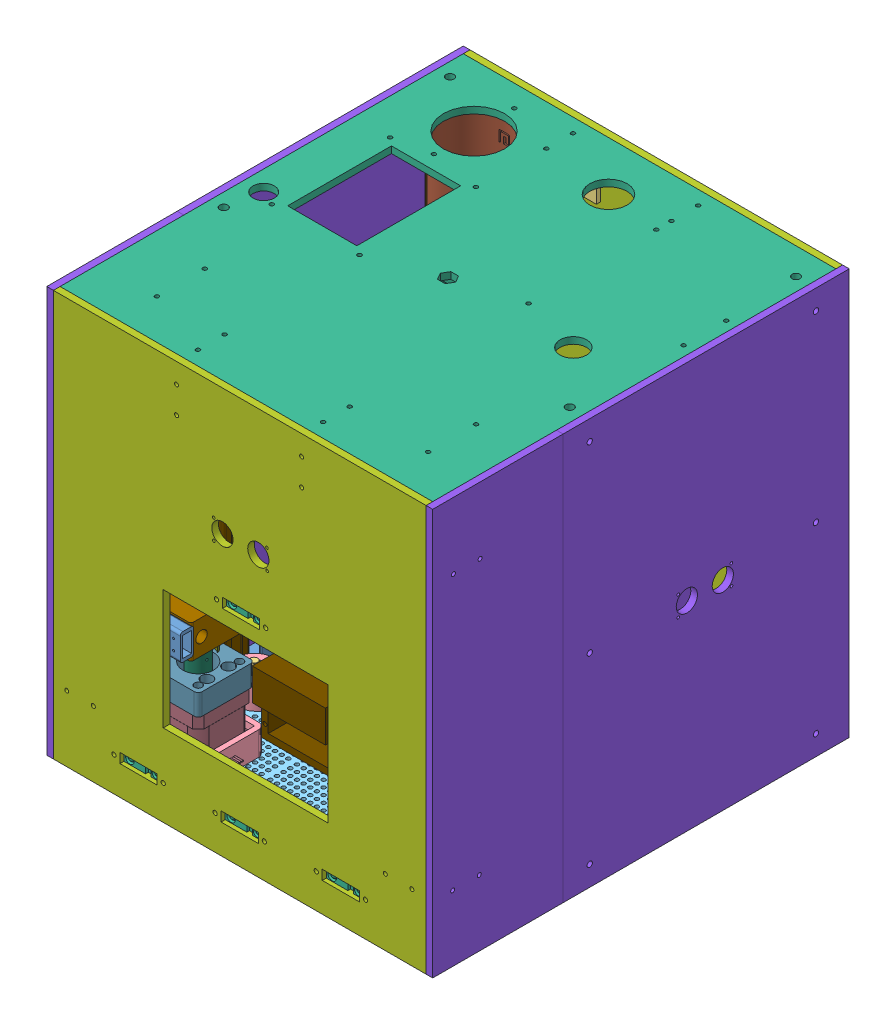
SolidWorks assembly Base_grand_robot_V3, configuration Défaut. Lengths in mm.
Overall size (315.25 345.84 313).
174 component instances, 54 part files, 167 mates.
Components (placement in the parent):
- base_v3-1: base_v3 [Défaut] at (-13.7179 5.8501 0) size (280 5 210)
- bille_porteuse-1: bille_porteuse [Défaut] at (91.4296 18.7222 119.3)
- bille_porteuse-3: bille_porteuse [Défaut] at (-113.9704 18.7222 119.3)
- bille_porteuse-4: bille_porteuse [Défaut] at (91.4296 18.7222 89.3)
- bloc moteur-1: bloc moteur [Défaut] at (-93.812 100.3945 0) size (96.7 249.86 114.05)
  - support moteur-1: support moteur [Défaut] at (-52.9059 10.4555 40) size (89 2 80)
  - support central-1: support central [Défaut] at (30.0941 -89.5445 40) size (6 100 80)
  - support inter-1: support inter [Défaut] at (-10.9059 -89.5445 40) size (6 100 80)
  - support exter-1: support exter [Défaut] at (-52.9059 -27.5445 40) x (-1 0 0) z (0 -1 0) size (6 80 25)
  - RENFORT-1: RENFORT [Défaut] at (-10.9059 -27.5445 -30) x (0 0 -1) z (1 0 0) size (10 38 42)
  - RENFORT-2: RENFORT [Défaut] at (-10.9059 -27.5445 40) x (0 0 -1) z (1 0 0) size (10 38 42)
  - fix carre-1: fix carre [Défaut] at (30.0941 -89.5445 0) x (0 0 -1) z (1 0 0) size (80 10 10)
  - fix carre-2: fix carre [Défaut] at (30.0941 0.4555 0) x (0 0 1) z (0 -1 0) size (80 10 10)
  - fix carre-3: fix carre [Défaut] at (-10.9059 -89.5445 0) x (0 0 -1) z (1 0 0) size (80 10 10)
  - moteur-1: moteur [Défaut] at (-31.9059 133.2945 0.001) x (-0.000071 0 -1) z (-1 0 0.000071) size (36.98 140.84 36.98)
  - support coulisse-1: support coulisse [Défaut] at (-48.9059 -11.0445 -20) x (1 0 0) z (0 1 0) size (28 10 10)
  - support coulisse-2: support coulisse [Défaut] at (-48.9059 -11.0445 30) x (1 0 0) z (0 1 0) size (28 10 10)
  - axe inter-1: axe inter [Défaut] at (36.0941 -12.5445 0) x (0 0.999221 -0.039455) z (-1 0 0) size (8 8 60)
  - axe roue-1: axe roue [Défaut] at (36.0941 -59.5445 0) x (0 0.572266 -0.820068) z (-1 0 0) size (8 8 50)
  - roue-1: roue [Défaut] at (5.7816 -59.5445 0) x (0 -0.770299 0.637683) z (0 -0.637683 -0.770299) size (81 21.5 81)
  - angular contact ball bearing_68_iso-6: angular contact ball bearing_68_iso [ISO 15 ABB - 288 - 12,SI,NC,12_68] at (-7.4059 -12.5445 0) size (5 16 16)
  - angular contact ball bearing_68_iso-7: angular contact ball bearing_68_iso [ISO 15 ABB - 288 - 12,SI,NC,12_68] at (33.5941 -59.5445 0) size (5 16 16)
  - angular contact ball bearing_68_iso-8: angular contact ball bearing_68_iso [ISO 15 ABB - 288 - 12,SI,NC,12_68] at (-55.4059 -12.5445 0) x (-1 0 0) z (0 0.924225 0.381849) size (5 16 16)
  - angular contact ball bearing_68_iso-9: angular contact ball bearing_68_iso [ISO 15 ABB - 288 - 12,SI,NC,12_68] at (-8.4059 -59.5445 0) size (5 16 16)
  - angular contact ball bearing_68_iso-10: angular contact ball bearing_68_iso [ISO 15 ABB - 288 - 12,SI,NC,12_68] at (33.5941 -12.5445 0) x (1 0 0) z (0 0.752289 -0.658833) size (5 16 16)
  - poulie 20 dents-1: poulie 20 dents [Défaut] at (19.2816 -12.5445 0) x (0 -0.673947 -0.73878) z (1 0 0) size (24 24 16.81)
  - poulie 30 dents-1: poulie 30 dents [Défaut] at (28.2816 -59.5445 0) x (0 -0.380704 -0.924697) z (-1 0 0) size (28.16 28.16 8)
  - Courroie2^bloc moteur-1: Courroie2^bloc moteur [Défaut] at (28.2816 -59.5445 0) x (0 0 -1) z (1 0 0) size (30.24 72.47 0) (virtual)
  - socket head cap screw_iso-1: socket head cap screw_iso [ISO 4762 M5 x 16 --- 16C] at (-47.9059 15.6555 35) x (0 -1 0) z (0.408943 0 0.91256) size (21 8.5 8.5)
  - socket head cap screw_iso-2: socket head cap screw_iso [ISO 4762 M5 x 16 --- 16C] at (-47.9059 15.6555 -35) x (0 -1 0) z (1 0 0) size (21 8.5 8.5)
  - socket head cap screw_iso-3: socket head cap screw_iso [ISO 4762 M5 x 16 --- 16C] at (-15.9059 15.6555 -35) x (0 -1 0) z (-0.986774 0 0.1621) size (21 8.5 8.5)
  - socket head cap screw_iso-4: socket head cap screw_iso [ISO 4762 M5 x 16 --- 16C] at (-15.9059 15.6555 35) x (0 -1 0) z (0 0 1) size (21 8.5 8.5)
  - socket head cap screw_iso-5: socket head cap screw_iso [ISO 4762 M6 x 10 --- 10C] at (25.0941 16.7055 -20) x (0 -1 0) z (0.924225 0 -0.381849) size (16 10 10)
  - socket head cap screw_iso-6: socket head cap screw_iso [ISO 4762 M6 x 10 --- 10C] at (25.0941 16.7055 20) x (0 -1 0) z (0 0 1) size (16 10 10)
  - socket head cap screw_iso-7: socket head cap screw_iso [ISO 4762 M6 x 16 --- 16C] at (-43.9059 -16.0445 -46.25) x (0 0 1) z (-1 0 0) size (22 10 10)
  - socket head cap screw_iso-8: socket head cap screw_iso [ISO 4762 M6 x 16 --- 16C] at (-25.9059 -16.0445 -46.25) x (0 0 1) z (-1 0 0) size (22 10 10)
  - socket head cap screw_iso-9: socket head cap screw_iso [ISO 4762 M6 x 16 --- 16C] at (-43.9059 -16.0445 46.25) x (0 0 -1) z (-0.381849 0.924225 0) size (22 10 10)
  - socket head cap screw_iso-10: socket head cap screw_iso [ISO 4762 M6 x 16 --- 16C] at (-25.9059 -16.0445 46.25) x (0 0 -1) z (0.987997 0.154474 0) size (22 10 10)
  - socket countersunk head screw_iso-1: socket countersunk head screw_iso [ISO 10642 - M5 x 16 --- 16N] at (-60.0059 -9.5445 35) x (1 0 0) z (0 -0.519107 0.854709) size (16 9.43 9.43)
  - socket countersunk head screw_iso-2: socket countersunk head screw_iso [ISO 10642 - M5 x 16 --- 16N] at (-60.0059 -22.5445 35) size (16 9.43 9.43)
  - socket countersunk head screw_iso-3: socket countersunk head screw_iso [ISO 10642 - M5 x 16 --- 16N] at (-60.0059 -22.5445 -35) size (16 9.43 9.43)
  - socket countersunk head screw_iso-4: socket countersunk head screw_iso [ISO 10642 - M5 x 16 --- 16N] at (-60.0059 -9.5445 -35) x (1 0 0) z (0 0.039879 0.999205) size (16 9.43 9.43)
  - socket countersunk head screw_iso-5: socket countersunk head screw_iso [ISO 10642 - M5 x 16 --- 16N] at (36.6941 5.4555 30) x (-1 0 0) z (0 0.924225 0.381849) size (16 9.43 9.43)
  - socket countersunk head screw_iso-6: socket countersunk head screw_iso [ISO 10642 - M5 x 16 --- 16N] at (36.6941 5.4555 -30) x (-1 0 0) z (0 0.924225 0.381849) size (16 9.43 9.43)
  - socket countersunk head screw_iso-7: socket countersunk head screw_iso [ISO 10642 - M5 x 16 --- 16N] at (36.6941 -84.5445 20) x (-1 0 0) z (0 0.924225 0.381849) size (16 9.43 9.43)
  - socket countersunk head screw_iso-8: socket countersunk head screw_iso [ISO 10642 - M5 x 16 --- 16N] at (36.6941 -84.5445 -20) x (-1 0 0) z (0 0.924225 0.381849) size (16 9.43 9.43)
  - socket countersunk head screw_iso-10: socket countersunk head screw_iso [ISO 10642 - M5 x 16 --- 16N] at (-4.3059 -84.5445 20) x (-1 0 0) z (0 0.924225 0.381849) size (16 9.43 9.43)
- bloc moteur-2: bloc moteur [Défaut] at (66.3761 100.3945 0) x (-1 0 0) z (0 0 -1) size (96.7 249.86 114.05)
  - support moteur-1: support moteur [Défaut] at (-52.9059 10.4555 40) size (89 2 80)
  - support central-1: support central [Défaut] at (30.0941 -89.5445 40) size (6 100 80)
  - support inter-1: support inter [Défaut] at (-10.9059 -89.5445 40) size (6 100 80)
  - support exter-1: support exter [Défaut] at (-52.9059 -27.5445 40) x (-1 0 0) z (0 -1 0) size (6 80 25)
  - RENFORT-1: RENFORT [Défaut] at (-10.9059 -27.5445 -30) x (0 0 -1) z (1 0 0) size (10 38 42)
  - RENFORT-2: RENFORT [Défaut] at (-10.9059 -27.5445 40) x (0 0 -1) z (1 0 0) size (10 38 42)
  - fix carre-1: fix carre [Défaut] at (30.0941 -89.5445 0) x (0 0 -1) z (1 0 0) size (80 10 10)
  - fix carre-2: fix carre [Défaut] at (30.0941 0.4555 0) x (0 0 1) z (0 -1 0) size (80 10 10)
  - fix carre-3: fix carre [Défaut] at (-10.9059 -89.5445 0) x (0 0 -1) z (1 0 0) size (80 10 10)
  - moteur-1: moteur [Défaut] at (-31.9059 133.2945 0.001) x (-0.000071 0 -1) z (-1 0 0.000071) size (36.98 140.84 36.98)
  - support coulisse-1: support coulisse [Défaut] at (-48.9059 -11.0445 -20) x (1 0 0) z (0 1 0) size (28 10 10)
  - support coulisse-2: support coulisse [Défaut] at (-48.9059 -11.0445 30) x (1 0 0) z (0 1 0) size (28 10 10)
  - axe inter-1: axe inter [Défaut] at (36.0941 -12.5445 0) x (0 0.999221 -0.039455) z (-1 0 0) size (8 8 60)
  - axe roue-1: axe roue [Défaut] at (36.0941 -59.5445 0) x (0 0.572266 -0.820068) z (-1 0 0) size (8 8 50)
  - roue-1: roue [Défaut] at (5.7816 -59.5445 0) x (0 -0.770299 0.637683) z (0 -0.637683 -0.770299) size (81 21.5 81)
  - angular contact ball bearing_68_iso-6: angular contact ball bearing_68_iso [ISO 15 ABB - 288 - 12,SI,NC,12_68] at (-7.4059 -12.5445 0) size (5 16 16)
  - angular contact ball bearing_68_iso-7: angular contact ball bearing_68_iso [ISO 15 ABB - 288 - 12,SI,NC,12_68] at (33.5941 -59.5445 0) size (5 16 16)
  - angular contact ball bearing_68_iso-8: angular contact ball bearing_68_iso [ISO 15 ABB - 288 - 12,SI,NC,12_68] at (-55.4059 -12.5445 0) x (-1 0 0) z (0 0.924225 0.381849) size (5 16 16)
  - angular contact ball bearing_68_iso-9: angular contact ball bearing_68_iso [ISO 15 ABB - 288 - 12,SI,NC,12_68] at (-8.4059 -59.5445 0) size (5 16 16)
  - angular contact ball bearing_68_iso-10: angular contact ball bearing_68_iso [ISO 15 ABB - 288 - 12,SI,NC,12_68] at (33.5941 -12.5445 0) x (1 0 0) z (0 0.752289 -0.658833) size (5 16 16)
  - poulie 20 dents-1: poulie 20 dents [Défaut] at (19.2816 -12.5445 0) x (0 -0.673947 -0.73878) z (1 0 0) size (24 24 16.81)
  - poulie 30 dents-1: poulie 30 dents [Défaut] at (28.2816 -59.5445 0) x (0 -0.380704 -0.924697) z (-1 0 0) size (28.16 28.16 8)
  - Courroie2^bloc moteur-1: Courroie2^bloc moteur [Défaut] at (28.2816 -59.5445 0) x (0 0 -1) z (1 0 0) size (30.24 72.47 0) (virtual)
  - socket head cap screw_iso-1: socket head cap screw_iso [ISO 4762 M5 x 16 --- 16C] at (-47.9059 15.6555 35) x (0 -1 0) z (0.408943 0 0.91256) size (21 8.5 8.5)
  - socket head cap screw_iso-2: socket head cap screw_iso [ISO 4762 M5 x 16 --- 16C] at (-47.9059 15.6555 -35) x (0 -1 0) z (1 0 0) size (21 8.5 8.5)
  - socket head cap screw_iso-3: socket head cap screw_iso [ISO 4762 M5 x 16 --- 16C] at (-15.9059 15.6555 -35) x (0 -1 0) z (-0.986774 0 0.1621) size (21 8.5 8.5)
  - socket head cap screw_iso-4: socket head cap screw_iso [ISO 4762 M5 x 16 --- 16C] at (-15.9059 15.6555 35) x (0 -1 0) z (0 0 1) size (21 8.5 8.5)
  - socket head cap screw_iso-5: socket head cap screw_iso [ISO 4762 M6 x 10 --- 10C] at (25.0941 16.7055 -20) x (0 -1 0) z (0.924225 0 -0.381849) size (16 10 10)
  - socket head cap screw_iso-6: socket head cap screw_iso [ISO 4762 M6 x 10 --- 10C] at (25.0941 16.7055 20) x (0 -1 0) z (0 0 1) size (16 10 10)
  - socket head cap screw_iso-7: socket head cap screw_iso [ISO 4762 M6 x 16 --- 16C] at (-43.9059 -16.0445 -46.25) x (0 0 1) z (-1 0 0) size (22 10 10)
  - socket head cap screw_iso-8: socket head cap screw_iso [ISO 4762 M6 x 16 --- 16C] at (-25.9059 -16.0445 -46.25) x (0 0 1) z (-1 0 0) size (22 10 10)
  - socket head cap screw_iso-9: socket head cap screw_iso [ISO 4762 M6 x 16 --- 16C] at (-43.9059 -16.0445 46.25) x (0 0 -1) z (-0.381849 0.924225 0) size (22 10 10)
  - socket head cap screw_iso-10: socket head cap screw_iso [ISO 4762 M6 x 16 --- 16C] at (-25.9059 -16.0445 46.25) x (0 0 -1) z (0.987997 0.154474 0) size (22 10 10)
  - socket countersunk head screw_iso-1: socket countersunk head screw_iso [ISO 10642 - M5 x 16 --- 16N] at (-60.0059 -9.5445 35) x (1 0 0) z (0 -0.519107 0.854709) size (16 9.43 9.43)
  - socket countersunk head screw_iso-2: socket countersunk head screw_iso [ISO 10642 - M5 x 16 --- 16N] at (-60.0059 -22.5445 35) size (16 9.43 9.43)
  - socket countersunk head screw_iso-3: socket countersunk head screw_iso [ISO 10642 - M5 x 16 --- 16N] at (-60.0059 -22.5445 -35) size (16 9.43 9.43)
  - socket countersunk head screw_iso-4: socket countersunk head screw_iso [ISO 10642 - M5 x 16 --- 16N] at (-60.0059 -9.5445 -35) x (1 0 0) z (0 0.039879 0.999205) size (16 9.43 9.43)
  - socket countersunk head screw_iso-5: socket countersunk head screw_iso [ISO 10642 - M5 x 16 --- 16N] at (36.6941 5.4555 30) x (-1 0 0) z (0 0.924225 0.381849) size (16 9.43 9.43)
  - socket countersunk head screw_iso-6: socket countersunk head screw_iso [ISO 10642 - M5 x 16 --- 16N] at (36.6941 5.4555 -30) x (-1 0 0) z (0 0.924225 0.381849) size (16 9.43 9.43)
  - socket countersunk head screw_iso-7: socket countersunk head screw_iso [ISO 10642 - M5 x 16 --- 16N] at (36.6941 -84.5445 20) x (-1 0 0) z (0 0.924225 0.381849) size (16 9.43 9.43)
  - socket countersunk head screw_iso-8: socket countersunk head screw_iso [ISO 10642 - M5 x 16 --- 16N] at (36.6941 -84.5445 -20) x (-1 0 0) z (0 0.924225 0.381849) size (16 9.43 9.43)
  - socket countersunk head screw_iso-10: socket countersunk head screw_iso [ISO 10642 - M5 x 16 --- 16N] at (-4.3059 -84.5445 20) x (-1 0 0) z (0 0.924225 0.381849) size (16 9.43 9.43)
- socket countersunk head screw_iso-10: socket countersunk head screw_iso [ISO 10642 - M5 x 16 --- 16N] at (82.2821 24.0329 -30) x (0 -1 0) z (-0.068023 0 0.997684) size (16 9.43 9.43)
- Profile-1: Profile [Défaut] at (-133.7179 310.8501 75) x (1 0 0) z (0 -1 0) size (20 20 300)
- Profile-2: Profile [Défaut] at (126.2821 310.8501 75) x (1 0 0) z (0 -1 0) size (20 20 300)
- bille-1: bille [Défaut] at (88.9821 9.4556 -89.3) size (14 14 14)
- porte_bille-1: porte_bille [Défaut] at (88.9821 9.4556 -89.3) size (16 1.79 16)
- contour_roulement-1: contour_roulement [Défaut] at (88.9821 22.8501 -89.3) x (0.737581 0 0.675259) z (-0.675259 0 0.737581) size (20 32.58 20)
- bille_porteuse-5: bille_porteuse [Défaut] at (-113.9704 18.7222 -119.3)
- Support_bille_appui-1: Support_bille_appui [Défaut] at (88.9821 10.8501 -89.3) x (0 0 1) z (-1 0 0) size (30 20 30)
- ecrou socket-1: ecrou socket [Défaut] at (88.9821 33.8501 -89.3) x (1 0 0) z (0 -1 0) size (12.41 10.75 3)
- ecrou socket-2: ecrou socket [Défaut] at (-116.4179 33.8501 89.3) x (1 0 0) z (0 -1 0) size (12.41 10.75 3)
- ecrou socket-3: ecrou socket [Défaut] at (-116.4179 33.8501 -89.3) x (1 0 0) z (0 -1 0) size (12.41 10.75 3)
- ecrou socket-4: ecrou socket [Défaut] at (88.9821 33.8501 89.3) x (1 0 0) z (0 -1 0) size (12.41 10.75 3)
- bille-2: bille [Défaut] at (-116.4179 9.4556 -89.3) size (14 14 14)
- bille-3: bille [Défaut] at (88.9821 9.4556 89.3) size (14 14 14)
- bille-4: bille [Défaut] at (-116.4179 9.4556 89.3) size (14 14 14)
- contour_roulement-2: contour_roulement [Défaut] at (-116.4179 21.8501 89.3) size (20 32.58 20)
- contour_roulement-3: contour_roulement [Défaut] at (-116.4179 21.8501 -89.3) size (20 32.58 20)
- contour_roulement-4: contour_roulement [Défaut] at (88.9821 21.8501 89.3) size (20 32.58 20)
- Support_bille_appui-2: Support_bille_appui [Défaut] at (-116.4179 10.8501 -89.3) size (30 20 30)
- Support_bille_appui-3: Support_bille_appui [Défaut] at (88.9821 10.8501 89.3) size (30 20 30)
- Support_bille_appui-4: Support_bille_appui [Défaut] at (-116.4179 10.8501 89.3) size (30 20 30)
- Profile-3: Profile [Défaut] at (-133.7179 310.8501 -95) x (1 0 0) z (0 -1 0) size (20 20 300)
- Profile-4: Profile [Défaut] at (126.2821 310.8501 -95) x (1 0 0) z (0 -1 0) size (20 20 300)
- porte_bille-2: porte_bille [Défaut] at (-116.4179 9.4556 -89.3) size (16 1.79 16)
- porte_bille-3: porte_bille [Défaut] at (-116.4179 9.4556 89.3) size (16 1.79 16)
- porte_bille-4: porte_bille [Défaut] at (88.9821 9.4556 89.3) size (16 1.79 16)
- support_haut_moteur-2: support_haut_moteur [Défaut] at (-153.7179 310.8501 105) x (1 0 0) z (0 1 0) size (280 303 5)
- Protege_arriere-1: Protege_arriere [Défaut] at (-153.7179 10.8501 -110) size (280 305 5)
- Protege_laterale_gauche-1: Protege_laterale_gauche [Défaut] at (131.2821 10.8501 -110) x (0 0 1) z (-1 0 0) size (313 305 5)
- Protege_laterale_gauche-2: Protege_laterale_gauche [Défaut] at (-158.7179 315.8501 -110) x (0 0 1) z (1 0 0) size (313 305 5)
- SUPPORT DU MILIEU-1: SUPPORT DU MILIEU [Défaut] at (-112.6768 236.5001 168.8547) x (0 0 1) z (0 -1 0) size (77 260.78 291)
  - support-milieu_droite-1: support-milieu_droite [Défaut] at (-88.6499 -39.4754 108.65) size (60 77 67.3)
  - support-milieu_gauche-1: support-milieu_gauche [Défaut] at (52.3501 -167.1754 108.65) x (-1 0 0) z (0 0 1) size (65 52.31 50)
  - poulie pour courroie-2: poulie pour courroie [Défaut] at (-30.6416 -209.3078 87.41) x (0 0.720856 -0.693085) z (-1 0 0) size (14 14 16)
  - roulement lineaire M8-24-1: roulement lineaire M8-24 [Défaut] at (-27.6499 -177.1754 109.65) size (15 15 24)
  - roulement lineaire M8-24-2: roulement lineaire M8-24 [Défaut] at (-11.3499 -177.1754 109.65) size (15 15 24)
  - roulement lineaire M8-24-3: roulement lineaire M8-24 [Défaut] at (3.3501 -113.5864 121.15) x (0.720875 0 -0.693065) z (0 1 0) size (15 15 24)
  - roulement lineaire M8-24-4: roulement lineaire M8-24 [Défaut] at (-40.6499 -113.5864 121.15) x (1 0 0) z (0 1 0) size (15 15 24)
  - roulement lineaire M8-24-5: roulement lineaire M8-24 [Défaut] at (-10.6499 -29.4754 109.65) size (15 15 24)
  - roulement lineaire M8-24-6: roulement lineaire M8-24 [Défaut] at (-26.9499 -29.4808 109.65) size (15 15 24)
  - moteur NEMA 17-40mm-2: moteur NEMA 17-40mm [Défaut] at (-18.8047 -14.8331 176.65) size (42.3 52.3 64)
  - moteur NEMA 17-40mm-3: moteur NEMA 17-40mm [Défaut] at (-19.4999 -191.8089 176.65) size (42.3 52.3 64)
  - support8moteur-1: support8moteur [Défaut] at (-39.9547 -35.9831 160.65) size (42.3 42.3 16)
  - support8moteur-2: support8moteur [Défaut] at (1.6501 -170.6589 160.65) x (-1 0 0) z (0 0 1) size (42.3 42.3 16)
  - Adaptateur-1: Adaptateur [Défaut] at (-18.1766 -22.3068 142.65) x (0 0 1) z (-0.996487 -0.083748 0) size (32 15 15)
  - Adaptateur-2: Adaptateur [Défaut] at (-21.6474 -198.9949 142.65) x (0 0 1) z (-0.95813 0.286335 0) size (32 15 15)
  - PINCE_ANTI_WOOBLE-1: PINCE_ANTI_WOOBLE [Défaut] at (-19.915 -24.8562 132.474) x (0.497684 -0.867358 0) z (0 0 1) size (29.81 20 10)
  - PINCE_ANTI_WOOBLE-2: PINCE_ANTI_WOOBLE [Défaut] at (-26.86 -198.7027 133.65) x (-0.185768 -0.982594 0) z (0 0 1) size (29.81 20 10)
  - support_haut-1: support_haut [Défaut] at (8.4901 -167.1639 -59.35) x (0 -1 0) z (0 0 -1) size (47.74 55.98 15)
  - support_haut-2: support_haut [Défaut] at (-46.7865 -39.4874 -59.35) x (-0.000332 1 0) z (0 0 -1) size (47.74 55.98 15)
  - moteur NEMA 17-40mm-4: moteur NEMA 17-40mm [Défaut] at (-28.6499 16.6746 87.5) x (0 1 0) z (1 0 0) size (42.3 52.3 64)
  - poulie pour courroie-3: poulie pour courroie [Défaut] at (-30.6499 16.6746 87.5) x (0 -0.523843 -0.851815) z (-1 0 0) size (14 14 16)
  - ENSEMBLE CHARIOT DEPLACEMENT_1-1: ENSEMBLE CHARIOT DEPLACEMENT_1 [Défaut] at (-40.172 -62.0864 90.8609) x (0 0 1) z (0 -1 0) size (95 70 55)
  - support_fin_de_coursz-1: support_fin_de_coursz [Défaut] at (21.3501 -6.4754 128.814) x (-1 0 0) z (0 -1 0) size (10 20 35)
  - support_fin_de_coursz-2: support_fin_de_coursz [Défaut] at (12.3501 -200.1754 128.65) x (1 0 0) z (0 1 0) size (10 20 35)
- socle00-1: socle00 [Défaut] at (-131.7179 15.8501 -105.2) x (1 0 0) z (0 -1 0) size (236 105.2 5)
- EQUERRE-1: EQUERRE [Défaut] at (43.2821 15.8501 -105.1) x (0 1 0) z (0 0 1) size (40 20 40)
- EQUERRE-2: EQUERRE [Défaut] at (-50.7179 15.8501 -105.1) x (0 1 0) z (0 0 1) size (40 20 40)
- EQUERRE-3: EQUERRE [Défaut] at (-70.7179 310.8501 -105) x (0 -1 0) z (0 0 1) size (40 20 40)
- EQUERRE-4: EQUERRE [Défaut] at (23.2821 310.8501 -105) x (0 -1 0) z (0 0 1) size (40 20 40)
- support moteur pas a pas-1: support moteur pas a pas [Default] at (104.2821 15.8501 124.9) x (-1 0 0) z (0 1 0) size (50.3 50.3 18)
- support moteur pas a pas-2: support moteur pas a pas [Default] at (-72.6937 15.8501 124.9) x (-1 0 0) z (0 1 0) size (50.3 50.3 18)
- socleV2-1: socleV2 [Default] at (-131.7179 10.8501 105.2) x (1 0 0) z (0 1 0) size (280 175.2 5)
- Ram Electronics Shop_IR Sensor_SHARP-10: Ram Electronics Shop_IR Sensor_SHARP [Default] at (-89.7679 36.4501 186.5) x (-1 0 0) z (0 1 0) size (44.5 13.5 17.1)
- Ram Electronics Shop_IR Sensor_SHARP-11: Ram Electronics Shop_IR Sensor_SHARP [Default] at (-13.7179 36.5501 186.5) x (-1 0 0) z (0 1 0) size (44.5 13.5 17.1)
- Ram Electronics Shop_IR Sensor_SHARP-12: Ram Electronics Shop_IR Sensor_SHARP [Default] at (-12.7679 176.0501 186.5) x (-1 0 0) z (0 1 0) size (44.5 13.5 17.1)
- Ram Electronics Shop_IR Sensor_SHARP-13: Ram Electronics Shop_IR Sensor_SHARP [Default] at (62.2821 36.4501 186.5) x (-1 0 0) z (0 1 0) size (44.5 13.5 17.1)
- Ram Electronics Shop_IR Sensor_SHARP-14: Ram Electronics Shop_IR Sensor_SHARP [Default] at (-12.7179 94.4501 -93.5) x (1 0 0) z (0 1 0) size (44.5 13.5 17.1)
- PROTEGE FACE-1: PROTEGE FACE [Défaut] at (-153.7179 315.8501 198) x (0 -1 0) z (0 0 1) size (305 280 5)
- EQUERRE-5: EQUERRE [Défaut] at (126.2821 70.8501 198) x (0 0 -1) z (-1 0 0) size (40 20 40)
- EQUERRE-6: EQUERRE [Défaut] at (-50.7179 310.8501 198) x (0 -1 0) z (0 0 -1) size (40 20 40)
- EQUERRE-7: EQUERRE [Défaut] at (43.2821 310.8501 198) x (0 -1 0) z (0 0 -1) size (40 20 40)
- EQUERRE-8: EQUERRE [Défaut] at (-153.7179 70.8501 198) x (1 0 0) z (0 0 -1) size (40 20 40)
- EQUERRE SOCLE DROIT-2: EQUERRE SOCLE DROIT [Défaut] at (108.2821 15.8501 95) x (0 0 1) z (0 1 0) size (40 18 40)
- EQUERRE SOCLE-3: EQUERRE SOCLE [Défaut] at (-151.7179 15.8501 95) x (0 0 1) z (0 1 0) size (40 18 40)
- support batterieV2-1: support batterieV2 [Défaut] at (-76.7179 65.8501 40) x (1 0 0) z (0 -1 0) size (55 33 50)
- Assemblage canon-1: Assemblage canon [Défaut] at (-82.9084 292.371 -53.9301) x (0.130304 0.034496 -0.990874) z (-0.411994 -0.907142 -0.08576) size (74.27 99.53 150.05)
  - canon-1: canon [Défaut] at (3.1077 -22.9568 -9.6387) x (0.991582 -0.098986 0.083473) z (-0.034496 0.419409 0.907142) size (66 50 75)
  - acroche-1: acroche [Default] at (-2.4259 -0.9797 74.2971) x (0.130304 0.901821 -0.411994) z (-0.034496 0.419409 0.907142) size (30 20 5)
  - la boule-1: la boule [Default] at (11.0512 -5.8572 54.3234) x (-0.574658 0.639446 0.510761) z (-0.657873 -0.732165 0.176459) size (40 40 40)
  - lanceur-1: lanceur [Défaut] at (0.5532 8.1004 57.5351) x (0.991582 -0.098986 0.083473) z (0.124804 0.902385 -0.412463) size (40 20.54 40)
  - servo moteur-1: servo moteur [Défaut] at (-9.2227 26.8629 69.9848) x (-0.130304 -0.901821 0.411994) z (-0.034496 0.419409 0.907142) size (54 20 48)
  - support servo moteur 1-1: support servo moteur 1 [Default] at (-5.4229 -10.5334 97.3404) x (-0.990874 0.103992 -0.08576) z (0.034496 -0.419409 -0.907142) size (20 9 22.55)
  - support moteur 2-1: support moteur 2 [Default] at (10.2843 28.5577 79.8643) x (-0.990874 0.103992 -0.08576) z (0.034496 -0.419409 -0.907142) size (20 22.3 22.55)
Mates (geometry in assembly coordinates):
- Coaxiale1: concentric aligned: cylinder of base_v3-1 through (-116.4179 10.8501 -89.3) axis (0 -1 0) radius 10.1; cylinder of Support_bille_appui-2 through (-116.4179 30.8501 -89.3) axis (0 -1 0) radius 15
- Coaxiale2: concentric aligned: cylinder of base_v3-1 through (-116.4179 10.8501 89.3) axis (0 -1 0) radius 10.1; cylinder of Support_bille_appui-4 through (-116.4179 30.8501 89.3) axis (0 -1 0) radius 15
- Coaxiale3: concentric aligned: cylinder of base_v3-1 through (88.9821 10.8501 89.3) axis (0 -1 0) radius 10.1; cylinder of Support_bille_appui-3 through (88.9821 30.8501 89.3) axis (0 -1 0) radius 15
- Coaxiale5: concentric aligned: cylinder of base_v3-1 through (-116.4179 10.8501 102) axis (0 -1 0) radius 1.5; cylinder of Support_bille_appui-4 through (-116.4179 18.8501 102) axis (0 -1 0) radius 1.5
- Coaxiale6: concentric aligned: cylinder of base_v3-1 through (-116.4179 10.8501 -76.6) axis (0 -1 0) radius 1.5; cylinder of Support_bille_appui-2 through (-116.4179 18.8501 -76.6) axis (0 -1 0) radius 1.5
- Coaxiale8: concentric aligned: cylinder of base_v3-1 through (88.9821 10.8501 102) axis (0 -1 0) radius 1.5; cylinder of Support_bille_appui-3 through (88.9821 18.8501 102) axis (0 -1 0) radius 1.5
- Coïncidente2: coincident aligned: plane of base_v3-1 through (-13.7179 10.8501 0) normal (0 1 0); circle of Support_bille_appui-2
- Coïncidente4: coincident aligned: plane of base_v3-1 through (-13.7179 10.8501 0) normal (0 1 0); circle of Support_bille_appui-3
- Coïncidente5: coincident aligned: plane of base_v3-1 through (-13.7179 10.8501 0) normal (0 1 0); circle of Support_bille_appui-4
- Coïncidente17: coincident aligned: circle of base_v3-1; circle of bloc moteur-1/fix carre-1
- Coïncidente18: coincident aligned: circle of base_v3-1; circle of bloc moteur-1/fix carre-3
- Coïncidente21: coincident aligned: circle of base_v3-1; circle of bloc moteur-2/fix carre-1
- Coïncidente22: coincident aligned: circle of base_v3-1; circle of bloc moteur-2/fix carre-3
- Coïncidente25: coincident anti-aligned: plane of bloc moteur-2/fix carre-3 through (77.2821 20.8501 -40) normal (0 1 0); circle of socket countersunk head screw_iso-10
- Coaxiale20: concentric aligned: cylinder of bloc moteur-2/fix carre-3 through (82.2821 10.8501 -30) axis (0 1 0) radius 3; cylinder of socket countersunk head screw_iso-10 through (82.2821 24.0329 -30) axis (0 1 0) radius 2.5
- Coaxiale21: concentric anti-aligned: cylinder of base_v3-1 through (116.2821 10.8501 85) axis (0 -1 0) radius 3; cylinder of Profile-2 through (116.2821 10.8501 85) axis (0 1 0) radius 1.5
- Coïncidente29: coincident anti-aligned: plane of base_v3-1 through (-13.7179 10.8501 0) normal (0 1 0); plane of Profile-2 through (126.2821 10.8501 75) normal (0 -1 0)
- Coaxiale22: concentric anti-aligned: cylinder of base_v3-1 through (-143.7179 10.8501 85) axis (0 -1 0) radius 3; cylinder of Profile-1 through (-143.7179 10.8501 85) axis (0 1 0) radius 1.5
- Coïncidente30: coincident anti-aligned: plane of base_v3-1 through (-13.7179 10.8501 0) normal (0 1 0); plane of Profile-1 through (-133.7179 10.8501 75) normal (0 -1 0)
- Coïncidente31: coincident aligned: plane of base_v3-1 through (-153.7179 10.8501 -95) normal (-1 0 0); plane of Profile-1 through (-153.7179 10.8501 75) normal (-1 0 0)
- Coaxiale23: concentric anti-aligned: cylinder of base_v3-1 through (88.9821 10.8501 -89.3) axis (0 -1 0) radius 10.1; cylinder of porte_bille-1 through (88.9821 9.4556 -89.3) axis (0 1 0) radius 8
- Coïncidente37: coincident anti-aligned: plane of base_v3-1 through (-13.7179 5.8501 0) normal (0 -1 0); plane of porte_bille-1 through (94.9821 5.8501 -89.3) normal (0 1 0)
- Coaxiale24: concentric: sphere of bille-1; sphere of porte_bille-1
- Coaxiale25: concentric anti-aligned: cylinder of base_v3-1 through (88.9821 10.8501 -89.3) axis (0 -1 0) radius 10.1; cylinder of contour_roulement-1 through (88.9821 20.8501 -89.3) axis (0 1 0) radius 10
- Coïncidente38: coincident anti-aligned: plane of porte_bille-1 through (94.9821 5.8501 -89.3) normal (0 1 0); plane of contour_roulement-1 through (88.9821 5.8501 -89.3) normal (0 -1 0)
- Coaxiale26: concentric anti-aligned: cylinder of contour_roulement-1 through (88.9821 20.8501 -89.3) axis (0 1 0) radius 10; cylinder of Support_bille_appui-1 through (88.9821 22.8501 -89.3) axis (0 -1 0) radius 10
- Coaxiale30: concentric aligned: cylinder of base_v3-1 through (88.9821 10.8501 -102) axis (0 -1 0) radius 1.5; cylinder of Support_bille_appui-1 through (88.9821 18.8501 -102) axis (0 -1 0) radius 1.5
- Coaxiale31: concentric aligned: cylinder of base_v3-1 through (76.2821 10.8501 -89.3) axis (0 -1 0) radius 1.5; cylinder of Support_bille_appui-1 through (76.2821 18.8501 -89.3) axis (0 -1 0) radius 1.5
- Coaxiale32: concentric anti-aligned: cylinder of contour_roulement-1 through (88.9821 37.8501 -89.3) axis (0 -1 0) radius 3; cylinder of ecrou socket-1 through (88.9821 30.8501 -89.3) axis (0 1 0) radius 3
- Coïncidente44: coincident anti-aligned: plane of base_v3-1 through (-13.7179 10.8501 0) normal (0 1 0); plane of Support_bille_appui-1 through (88.9821 10.8501 -89.3) normal (0 -1 0)
- Coïncidente45: coincident anti-aligned: plane of Support_bille_appui-1 through (88.9821 30.8501 -89.3) normal (0 1 0); plane of ecrou socket-1 through (88.9821 30.8501 -89.3) normal (0 -1 0)
- Coaxiale33: concentric anti-aligned: cylinder of base_v3-1 through (-116.4179 10.8501 -119.3) axis (0 -1 0) radius 10.1; cylinder of ? through (-116.4179 9.4556 -119.3) axis (0 1 0) radius 8
- Coïncidente46: coincident anti-aligned: plane of base_v3-1 through (-13.7179 5.8501 0) normal (0 -1 0); plane of ? through (-110.4179 5.8501 -119.3) normal (0 1 0)
- Coaxiale39: concentric: sphere of ?; sphere of bille-2
- Coaxiale40: concentric anti-aligned: cylinder of base_v3-1 through (-116.4179 10.8501 -89.3) axis (0 -1 0) radius 10.1; cylinder of contour_roulement-3 through (-116.4179 19.8501 -89.3) axis (0 1 0) radius 10
- Coïncidente50: coincident aligned: plane of ? through (-108.4179 4.8501 -119.3) normal (0 -1 0); plane of contour_roulement-3 through (-116.4179 4.8501 -119.3) normal (0 -1 0)
- Coaxiale41: concentric anti-aligned: cylinder of base_v3-1 through (-116.4179 10.8501 119.3) axis (0 -1 0) radius 10.1; cylinder of ? through (-116.4179 9.4556 119.3) axis (0 1 0) radius 8
- Coïncidente51: coincident anti-aligned: plane of base_v3-1 through (-13.7179 5.8501 0) normal (0 -1 0); plane of ? through (-110.4179 5.8501 119.3) normal (0 1 0)
- Coaxiale42: concentric: sphere of ?; sphere of bille-4
- Coaxiale43: concentric aligned: cylinder of base_v3-1 through (-116.4179 10.8501 89.3) axis (0 -1 0) radius 10.1; cylinder of Support_bille_appui-4 through (-116.4179 22.8501 89.3) axis (0 -1 0) radius 10
- Coaxiale44: concentric anti-aligned: cylinder of base_v3-1 through (-116.4179 10.8501 89.3) axis (0 -1 0) radius 10.1; cylinder of contour_roulement-2 through (-116.4179 4.8501 89.3) axis (0 1 0) radius 8
- Coïncidente54: coincident aligned: plane of ? through (-108.4179 4.8501 119.3) normal (0 -1 0); plane of contour_roulement-2 through (-116.4179 4.8501 119.3) normal (0 -1 0)
- Coaxiale45: concentric anti-aligned: cylinder of ecrou socket-2 through (-116.4179 30.8501 89.3) axis (0 1 0) radius 3; cylinder of contour_roulement-2 through (-116.4179 36.8501 89.3) axis (0 -1 0) radius 3
- Coaxiale46: concentric anti-aligned: cylinder of ecrou socket-3 through (-116.4179 30.8501 -89.3) axis (0 1 0) radius 3; cylinder of contour_roulement-3 through (-116.4179 36.8501 -89.3) axis (0 -1 0) radius 3
- Coaxiale47: concentric anti-aligned: cylinder of contour_roulement-3 through (-116.4179 19.8501 -89.3) axis (0 1 0) radius 10; cylinder of Support_bille_appui-2 through (-116.4179 30.8501 -89.3) axis (0 -1 0) radius 15
- Coaxiale48: concentric aligned: cylinder of base_v3-1 through (-116.4179 10.8501 -102) axis (0 -1 0) radius 1.5; cylinder of Support_bille_appui-2 through (-116.4179 18.8501 -102) axis (0 -1 0) radius 1.5
- Coaxiale49: concentric aligned: cylinder of base_v3-1 through (-103.7179 10.8501 -89.3) axis (0 -1 0) radius 1.5; cylinder of Support_bille_appui-2 through (-103.7179 18.8501 -89.3) axis (0 -1 0) radius 1.5
- Coïncidente55: coincident anti-aligned: plane of base_v3-1 through (-13.7179 10.8501 0) normal (0 1 0); plane of Support_bille_appui-2 through (-116.4179 10.8501 -89.3) normal (0 -1 0)
- Coïncidente56: coincident anti-aligned: plane of ecrou socket-3 through (-116.4179 30.8501 -89.3) normal (0 -1 0); plane of Support_bille_appui-2 through (-116.4179 30.8501 -89.3) normal (0 1 0)
- Coaxiale50: concentric aligned: cylinder of base_v3-1 through (-103.7179 10.8501 89.3) axis (0 -1 0) radius 1.5; cylinder of Support_bille_appui-4 through (-103.7179 18.8501 89.3) axis (0 -1 0) radius 1.5
- Coaxiale51: concentric aligned: cylinder of base_v3-1 through (-116.4179 10.8501 76.6) axis (0 -1 0) radius 1.5; cylinder of Support_bille_appui-4 through (-116.4179 18.8501 76.6) axis (0 -1 0) radius 1.5
- Coïncidente57: coincident anti-aligned: plane of base_v3-1 through (-13.7179 10.8501 0) normal (0 1 0); plane of Support_bille_appui-4 through (-116.4179 10.8501 89.3) normal (0 -1 0)
- Coïncidente58: coincident anti-aligned: plane of ecrou socket-2 through (-116.4179 30.8501 89.3) normal (0 -1 0); plane of Support_bille_appui-4 through (-116.4179 30.8501 89.3) normal (0 1 0)
- Coaxiale52: concentric anti-aligned: cylinder of base_v3-1 through (88.9821 10.8501 119.3) axis (0 -1 0) radius 10.1; cylinder of ? through (88.9821 9.4556 119.3) axis (0 1 0) radius 8
- Coïncidente59: coincident anti-aligned: plane of base_v3-1 through (-13.7179 5.8501 0) normal (0 -1 0); plane of ? through (94.9821 5.8501 119.3) normal (0 1 0)
- Coaxiale53: concentric: sphere of ?; sphere of bille-3
- Coaxiale54: concentric anti-aligned: cylinder of base_v3-1 through (88.9821 10.8501 89.3) axis (0 -1 0) radius 10.1; cylinder of contour_roulement-4 through (88.9821 19.8501 89.3) axis (0 1 0) radius 10
- Coïncidente60: coincident aligned: plane of ? through (96.9821 4.8501 119.3) normal (0 -1 0); plane of contour_roulement-4 through (88.9821 4.8501 119.3) normal (0 -1 0)
- Coaxiale55: concentric anti-aligned: cylinder of contour_roulement-4 through (88.9821 19.8501 89.3) axis (0 1 0) radius 10; cylinder of Support_bille_appui-3 through (88.9821 30.8501 89.3) axis (0 -1 0) radius 15
- Coaxiale56: concentric aligned: cylinder of base_v3-1 through (76.2821 10.8501 89.3) axis (0 -1 0) radius 1.5; cylinder of Support_bille_appui-3 through (76.2821 18.8501 89.3) axis (0 -1 0) radius 1.5
- Coaxiale57: concentric aligned: cylinder of base_v3-1 through (88.9821 10.8501 102) axis (0 -1 0) radius 1.5; cylinder of Support_bille_appui-3 through (88.9821 18.8501 102) axis (0 -1 0) radius 1.5
- Coaxiale58: concentric anti-aligned: cylinder of ecrou socket-4 through (88.9821 30.8501 89.3) axis (0 1 0) radius 3; cylinder of contour_roulement-4 through (88.9821 36.8501 89.3) axis (0 -1 0) radius 3
- Coïncidente62: coincident anti-aligned: plane of base_v3-1 through (-13.7179 10.8501 0) normal (0 1 0); plane of Support_bille_appui-3 through (88.9821 10.8501 89.3) normal (0 -1 0)
- Coïncidente63: coincident anti-aligned: plane of ecrou socket-4 through (88.9821 30.8501 89.3) normal (0 -1 0); plane of Support_bille_appui-3 through (88.9821 30.8501 89.3) normal (0 1 0)
- Coaxiale59: concentric anti-aligned: cylinder of base_v3-1 through (-143.7179 10.8501 -85) axis (0 -1 0) radius 3; cylinder of Profile-3 through (-143.7179 10.8501 -85) axis (0 1 0) radius 1.5
- Coïncidente64: coincident aligned: plane of base_v3-1 through (-153.7179 10.8501 -95) normal (-1 0 0); plane of Profile-3 through (-153.7179 10.8501 -95) normal (-1 0 0)
- Coïncidente65: coincident anti-aligned: plane of base_v3-1 through (-13.7179 10.8501 0) normal (0 1 0); plane of Profile-3 through (-133.7179 10.8501 -95) normal (0 -1 0)
- Coaxiale60: concentric anti-aligned: cylinder of base_v3-1 through (116.2821 10.8501 -85) axis (0 -1 0) radius 3; cylinder of Profile-4 through (116.2821 10.8501 -85) axis (0 1 0) radius 1.5
- Coïncidente66: coincident aligned: plane of base_v3-1 through (126.2821 10.8501 -95) normal (1 0 0); plane of Profile-4 through (126.2821 10.8501 -95) normal (1 0 0)
- Coïncidente67: coincident anti-aligned: plane of base_v3-1 through (-13.7179 10.8501 0) normal (0 1 0); plane of Profile-4 through (126.2821 10.8501 -95) normal (0 -1 0)
- Coaxiale64: concentric: sphere of bille-3; sphere of porte_bille-4
- Coaxiale65: concentric aligned: cylinder of contour_roulement-4 through (88.9821 4.8501 89.3) axis (0 1 0) radius 8; cylinder of porte_bille-4 through (88.9821 9.4556 89.3) axis (0 1 0) radius 8
- Coïncidente73: coincident anti-aligned: plane of base_v3-1 through (-13.7179 5.8501 0) normal (0 -1 0); plane of porte_bille-4 through (94.9821 5.8501 89.3) normal (0 1 0)
- Coaxiale66: concentric: sphere of bille-4; sphere of porte_bille-3
- Coaxiale67: concentric aligned: cylinder of contour_roulement-2 through (-116.4179 4.8501 89.3) axis (0 1 0) radius 8; cylinder of porte_bille-3 through (-116.4179 9.4556 89.3) axis (0 1 0) radius 8
- Coïncidente74: coincident anti-aligned: plane of base_v3-1 through (-13.7179 5.8501 0) normal (0 -1 0); plane of porte_bille-3 through (-110.4179 5.8501 89.3) normal (0 1 0)
- Coaxiale68: concentric: sphere of bille-2; sphere of porte_bille-2
- Coaxiale69: concentric aligned: cylinder of contour_roulement-3 through (-116.4179 4.8501 -89.3) axis (0 1 0) radius 8; cylinder of porte_bille-2 through (-116.4179 9.4556 -89.3) axis (0 1 0) radius 8
- Coïncidente75: coincident anti-aligned: plane of base_v3-1 through (-13.7179 5.8501 0) normal (0 -1 0); plane of porte_bille-2 through (-110.4179 5.8501 -89.3) normal (0 1 0)
- Coaxiale74: concentric anti-aligned: cylinder of Profile-2 through (116.2821 10.8501 85) axis (0 1 0) radius 1.5; cylinder of support_haut_moteur-2 through (116.2821 315.8501 85) axis (0 -1 0) radius 3
- Parallèle2: parallel anti-aligned: cylinder of Profile-4 through (116.2821 10.8501 -85) axis (0 1 0) radius 1.5; cylinder of support_haut_moteur-2 through (116.2821 315.8501 -85) axis (0 -1 0) radius 3
- Coaxiale77: concentric anti-aligned: cylinder of Profile-1 through (-143.7179 10.8501 85) axis (0 1 0) radius 1.5; cylinder of support_haut_moteur-2 through (-143.7179 315.8501 85) axis (0 -1 0) radius 3
- Coïncidente111: coincident aligned: plane of base_v3-1 through (126.2821 10.8501 -95) normal (1 0 0); plane of Profile-2 through (126.2821 10.8501 75) normal (1 0 0)
- Coïncidente120: coincident aligned: plane of Profile-4 through (126.2821 10.8501 -95) normal (1 0 0); plane of Protege_arriere-1 through (126.2821 10.8501 -105) normal (1 0 0)
- Coïncidente122: coincident anti-aligned: plane of base_v3-1 through (-13.7179 10.8501 0) normal (0 1 0); plane of Protege_arriere-1 through (-153.7179 10.8501 -105) normal (0 -1 0)
- Coïncidente125: coincident aligned: plane of Protege_arriere-1 through (-153.7179 10.8501 -110) normal (0 0 -1); plane of Protege_laterale_gauche-1 through (126.2821 10.8501 -110) normal (0 0 -1)
- Coïncidente126: coincident aligned: plane of support_haut_moteur-2 through (-153.7179 315.8501 105) normal (0 1 0); plane of Protege_laterale_gauche-1 through (126.2821 315.8501 -110) normal (0 1 0)
- Coïncidente136: coincident anti-aligned: plane of Protege_arriere-1 through (126.2821 10.8501 -105) normal (1 0 0); plane of Protege_laterale_gauche-1 through (126.2821 10.8501 -110) normal (-1 0 0)
- Coïncidente137: coincident aligned: plane of Protege_arriere-1 through (-153.7179 10.8501 -110) normal (0 0 -1); plane of Protege_laterale_gauche-2 through (-153.7179 315.8501 -110) normal (0 0 -1)
- Coïncidente138: coincident aligned: plane of support_haut_moteur-2 through (-153.7179 315.8501 105) normal (0 1 0); plane of Protege_laterale_gauche-2 through (-153.7179 315.8501 -110) normal (0 1 0)
- Coïncidente139: coincident anti-aligned: plane of support_haut_moteur-2 through (-153.7179 315.8501 105) normal (-1 0 0); plane of Protege_laterale_gauche-2 through (-153.7179 315.8501 -110) normal (1 0 0)
- Coïncidente141: coincident anti-aligned: plane of bloc moteur-1/support central-1 through (-57.7179 110.8501 40) normal (1 0 0); plane of socle00-1 through (-57.7179 10.8501 -105.2) normal (-1 0 0)
- Coïncidente147: coincident anti-aligned: plane of socle00-1 through (-131.7179 15.8501 -105.2) normal (0 1 0); plane of EQUERRE-1 through (43.2821 15.8501 -102.1) normal (0 -1 0)
- Coaxiale83: concentric anti-aligned: cylinder of socle00-1 through (33.2821 10.8501 -94.5) axis (0 1 0) radius 1.5; cylinder of EQUERRE-1 through (33.2821 18.8501 -94.5) axis (0 -1 0) radius 1.5
- Parallèle10: parallel aligned: plane of socle00-1 through (-131.7179 10.8501 -105.2) normal (0 0 -1); plane of EQUERRE-1 through (43.2821 15.8501 -105.1) normal (0 0 -1)
- Coïncidente149: coincident anti-aligned: plane of socle00-1 through (-131.7179 15.8501 -105.2) normal (0 1 0); plane of EQUERRE-2 through (-50.7179 15.8501 -102.1) normal (0 -1 0)
- Coaxiale84: concentric anti-aligned: cylinder of socle00-1 through (-60.7179 10.8501 -74.5) axis (0 1 0) radius 1.5; cylinder of EQUERRE-2 through (-60.7179 18.8501 -74.5) axis (0 -1 0) radius 1.5
- Parallèle11: parallel aligned: plane of socle00-1 through (-131.7179 10.8501 -105.2) normal (0 0 -1); plane of EQUERRE-2 through (-50.7179 15.8501 -105.1) normal (0 0 -1)
- Coïncidente151: coincident anti-aligned: plane of support_haut_moteur-2 through (-153.7179 310.8501 105) normal (0 -1 0); plane of EQUERRE-3 through (-70.7179 310.8501 -102) normal (0 1 0)
- Coïncidente152: coincident aligned: plane of support_haut_moteur-2 through (-153.7179 315.8501 -105) normal (0 0 -1); plane of EQUERRE-3 through (-70.7179 310.8501 -105) normal (0 0 -1)
- Coïncidente154: coincident aligned: plane of EQUERRE-2 through (-70.7179 15.8501 -102.1) normal (-1 0 0); plane of EQUERRE-3 through (-70.7179 310.8501 -102) normal (-1 0 0)
- Coïncidente155: coincident anti-aligned: plane of support_haut_moteur-2 through (-153.7179 310.8501 105) normal (0 -1 0); plane of EQUERRE-4 through (23.2821 310.8501 -102) normal (0 1 0)
- Coïncidente156: coincident aligned: plane of support_haut_moteur-2 through (-153.7179 315.8501 -105) normal (0 0 -1); plane of EQUERRE-4 through (23.2821 310.8501 -105) normal (0 0 -1)
- Coïncidente157: coincident aligned: plane of EQUERRE-1 through (43.2821 15.8501 -102.1) normal (1 0 0); plane of EQUERRE-4 through (43.2821 310.8501 -102) normal (1 0 0)
- Coïncidente158: coincident anti-aligned: plane of support_haut_moteur-2 through (-153.7179 315.8501 -105) normal (0 0 -1); plane of Protege_arriere-1 through (-153.7179 10.8501 -105) normal (0 0 1)
- Coïncidente159: coincident anti-aligned: plane of base_v3-1 through (-13.7179 10.8501 0) normal (0 1 0); plane of socleV2-1 through (-131.7179 10.8501 105.2) normal (0 -1 0)
- Coïncidente160: coincident anti-aligned: plane of bloc moteur-1/support central-1 through (-57.7179 110.8501 40) normal (1 0 0); plane of socleV2-1 through (-57.7179 15.8501 105.2) normal (-1 0 0)
- Coïncidente163: coincident anti-aligned: plane of bloc moteur-2/support central-1 through (30.2821 110.8501 -40) normal (-1 0 0); plane of socleV2-1 through (30.2821 15.8501 105.2) normal (1 0 0)
- Coïncidente164: coincident anti-aligned: plane of bloc moteur-1/fix carre-1 through (-73.7179 20.8501 40) normal (0 0 1); plane of socleV2-1 through (-131.7179 15.8501 40) normal (0 0 -1)
- Coïncidente170: coincident anti-aligned: plane of support moteur pas a pas-1 through (104.2821 15.8501 124.9) normal (0 -1 0); plane of socleV2-1 through (-131.7179 15.8501 105.2) normal (0 1 0)
- Coïncidente174: coincident aligned: plane of support moteur pas a pas-1 through (104.2821 19.8501 175.2) normal (0 0 1); plane of socleV2-1 through (-131.7179 15.8501 175.2) normal (0 0 1)
- Coïncidente176: coincident aligned: plane of support moteur pas a pas-2 through (-72.6937 19.8501 175.2) normal (0 0 1); plane of socleV2-1 through (-131.7179 15.8501 175.2) normal (0 0 1)
- Coïncidente179: coincident anti-aligned: plane of support moteur pas a pas-2 through (-72.6937 15.8501 124.9) normal (0 -1 0); plane of socleV2-1 through (-131.7179 15.8501 105.2) normal (0 1 0)
- Coïncidente183: coincident anti-aligned: plane of SUPPORT DU MILIEU-1/moteur NEMA 17-40mm-2 through (-118.9937 19.8501 133.0869) normal (-1 0 0); plane of support moteur pas a pas-2 through (-118.9937 33.8501 171.2) normal (1 0 0)
- Coïncidente184: coincident anti-aligned: plane of SUPPORT DU MILIEU-1/moteur NEMA 17-40mm-2 through (-114.8068 19.8501 171.2) normal (0 0 1); plane of support moteur pas a pas-2 through (-76.6937 33.8501 171.2) normal (0 0 -1)
- Coïncidente185: coincident anti-aligned: plane of SUPPORT DU MILIEU-1/moteur NEMA 17-40mm-2 through (-97.8437 19.8501 111.9369) normal (0 -1 0); plane of support moteur pas a pas-2 through (-72.6937 19.8501 124.9) normal (0 1 0)
- Coïncidente188: coincident anti-aligned: plane of SUPPORT DU MILIEU-1/moteur NEMA 17-40mm-3 through (100.2821 19.8501 132.3918) normal (1 0 0); plane of support moteur pas a pas-1 through (100.2821 33.8501 171.2) normal (-1 0 0)
- Coïncidente189: coincident anti-aligned: plane of Protege_laterale_gauche-1 through (126.2821 10.8501 -110) normal (-1 0 0); plane of PROTEGE FACE-1 through (126.2821 315.8501 203) normal (1 0 0)
- Coïncidente190: coincident anti-aligned: plane of Protege_laterale_gauche-2 through (-153.7179 315.8501 -110) normal (1 0 0); plane of PROTEGE FACE-1 through (-153.7179 315.8501 203) normal (-1 0 0)
- Coïncidente191: coincident aligned: plane of support_haut_moteur-2 through (-153.7179 315.8501 105) normal (0 1 0); plane of PROTEGE FACE-1 through (-153.7179 315.8501 203) normal (0 1 0)
- Coïncidente196: coincident anti-aligned: plane of support_haut_moteur-2 through (-153.7179 310.8501 105) normal (0 -1 0); plane of EQUERRE-7 through (43.2821 310.8501 195) normal (0 1 0)
- Coïncidente197: coincident aligned: plane of support_haut_moteur-2 through (126.2821 315.8501 198) normal (0 0 1); plane of EQUERRE-7 through (43.2821 310.8501 198) normal (0 0 1)
- Coïncidente198: coincident aligned: plane of EQUERRE-4 through (43.2821 310.8501 -102) normal (1 0 0); plane of EQUERRE-7 through (43.2821 310.8501 195) normal (1 0 0)
- Coïncidente199: coincident anti-aligned: plane of support_haut_moteur-2 through (-153.7179 310.8501 105) normal (0 -1 0); plane of EQUERRE-6 through (-50.7179 310.8501 195) normal (0 1 0)
- Coïncidente200: coincident aligned: plane of EQUERRE-3 through (-70.7179 310.8501 -102) normal (-1 0 0); plane of EQUERRE-6 through (-70.7179 310.8501 195) normal (-1 0 0)
- Coïncidente201: coincident aligned: plane of support_haut_moteur-2 through (126.2821 315.8501 198) normal (0 0 1); plane of EQUERRE-6 through (-50.7179 310.8501 198) normal (0 0 1)
- Coïncidente210: coincident anti-aligned: plane of Protege_laterale_gauche-2 through (-153.7179 315.8501 -110) normal (1 0 0); plane of EQUERRE-8 through (-153.7179 70.8501 195) normal (-1 0 0)
- Parallèle14: parallel anti-aligned: plane of support_haut_moteur-2 through (-153.7179 310.8501 105) normal (0 -1 0); plane of EQUERRE-8 through (-153.7179 70.8501 195) normal (0 1 0)
- Coïncidente212: coincident aligned: plane of support_haut_moteur-2 through (126.2821 315.8501 198) normal (0 0 1); plane of EQUERRE-8 through (-153.7179 70.8501 198) normal (0 0 1)
- Distance8: distance = 240 mm anti-aligned: plane of EQUERRE-8 through (-153.7179 70.8501 195) normal (0 1 0); plane of support_haut_moteur-2 through (-153.7179 310.8501 105) normal (0 -1 0)
- Coïncidente215: coincident anti-aligned: plane of Protege_laterale_gauche-1 through (126.2821 10.8501 -110) normal (-1 0 0); plane of EQUERRE-5 through (126.2821 70.8501 198) normal (1 0 0)
- Parallèle16: parallel anti-aligned: plane of support_haut_moteur-2 through (-153.7179 310.8501 105) normal (0 -1 0); plane of EQUERRE-5 through (123.2821 70.8501 198) normal (0 1 0)
- Coïncidente217: coincident aligned: plane of support_haut_moteur-2 through (126.2821 315.8501 198) normal (0 0 1); plane of EQUERRE-5 through (123.2821 70.8501 198) normal (0 0 1)
- Distance9: distance = 240 mm anti-aligned: plane of EQUERRE-5 through (123.2821 70.8501 198) normal (0 1 0); plane of support_haut_moteur-2 through (-153.7179 310.8501 105) normal (0 -1 0)
- Coïncidente222: coincident anti-aligned: plane of Ram Electronics Shop_IR Sensor_SHARP-10 through (-103.7179 40.0501 200) normal (-1 0 0); plane of PROTEGE FACE-1 through (-103.7179 40.1501 198) normal (1 0 0)
- Coïncidente223: coincident anti-aligned: plane of Ram Electronics Shop_IR Sensor_SHARP-10 through (-75.7679 32.8501 200) normal (0 -1 0); plane of PROTEGE FACE-1 through (-103.7179 32.8501 198) normal (0 1 0)
- Coïncidente224: coincident anti-aligned: plane of Ram Electronics Shop_IR Sensor_SHARP-10 through (-89.7679 36.4501 198) normal (0 0 1); plane of PROTEGE FACE-1 through (-153.7179 315.8501 198) normal (0 0 -1)
- Coïncidente225: coincident anti-aligned: plane of Ram Electronics Shop_IR Sensor_SHARP-11 through (0.2821 40.1501 200) normal (0 1 0); plane of PROTEGE FACE-1 through (-27.7179 40.1501 198) normal (0 -1 0)
- Coïncidente226: coincident anti-aligned: plane of Ram Electronics Shop_IR Sensor_SHARP-11 through (0.2821 40.1501 200) normal (1 0 0); plane of PROTEGE FACE-1 through (0.2821 40.1501 198) normal (-1 0 0)
- Coïncidente227: coincident anti-aligned: plane of Ram Electronics Shop_IR Sensor_SHARP-11 through (-13.7179 36.5501 198) normal (0 0 1); plane of PROTEGE FACE-1 through (-153.7179 315.8501 198) normal (0 0 -1)
- Coïncidente228: coincident anti-aligned: plane of Ram Electronics Shop_IR Sensor_SHARP-13 through (76.2821 32.8501 200) normal (0 -1 0); plane of PROTEGE FACE-1 through (48.2821 32.8501 198) normal (0 1 0)
- Coïncidente229: coincident anti-aligned: plane of Ram Electronics Shop_IR Sensor_SHARP-13 through (76.2821 40.0501 200) normal (1 0 0); plane of PROTEGE FACE-1 through (76.2821 40.1501 198) normal (-1 0 0)
- Coïncidente230: coincident anti-aligned: plane of Ram Electronics Shop_IR Sensor_SHARP-13 through (62.2821 36.4501 198) normal (0 0 1); plane of PROTEGE FACE-1 through (-153.7179 315.8501 198) normal (0 0 -1)
- Coïncidente231: coincident anti-aligned: plane of Ram Electronics Shop_IR Sensor_SHARP-12 through (1.2321 179.6501 200) normal (0 1 0); plane of PROTEGE FACE-1 through (-26.7179 179.6501 198) normal (0 -1 0)
- Coïncidente232: coincident anti-aligned: plane of Ram Electronics Shop_IR Sensor_SHARP-12 through (-26.7179 179.6501 200) normal (-1 0 0); plane of PROTEGE FACE-1 through (-26.7179 179.6501 198) normal (1 0 0)
- Coïncidente233: coincident anti-aligned: plane of Ram Electronics Shop_IR Sensor_SHARP-12 through (-12.7679 176.0501 198) normal (0 0 1); plane of PROTEGE FACE-1 through (-153.7179 315.8501 198) normal (0 0 -1)
- Coïncidente234: coincident anti-aligned: plane of Protege_arriere-1 through (1.2821 90.8501 -105) normal (0 1 0); plane of Ram Electronics Shop_IR Sensor_SHARP-14 through (-15.0679 90.8501 -107) normal (0 -1 0)
- Coïncidente236: coincident anti-aligned: plane of Protege_arriere-1 through (-26.7179 98.1501 -105) normal (1 0 0); plane of Ram Electronics Shop_IR Sensor_SHARP-14 through (-26.7179 98.0501 -107) normal (-1 0 0)
- Coïncidente237: coincident anti-aligned: plane of Protege_arriere-1 through (-153.7179 10.8501 -105) normal (0 0 1); plane of Ram Electronics Shop_IR Sensor_SHARP-14 through (-12.7179 94.4501 -105) normal (0 0 -1)
- Coïncidente249: coincident anti-aligned: plane of Profile-2 through (126.2821 10.8501 95) normal (0 0 1); plane of EQUERRE SOCLE DROIT-2 through (108.2821 18.8501 95) normal (0 0 -1)
- Coïncidente250: coincident anti-aligned: plane of socleV2-1 through (-131.7179 15.8501 105.2) normal (0 1 0); plane of EQUERRE SOCLE DROIT-2 through (108.2821 15.8501 95) normal (0 -1 0)
- Coïncidente252: coincident anti-aligned: plane of Protege_laterale_gauche-1 through (126.2821 10.8501 -110) normal (-1 0 0); plane of EQUERRE SOCLE DROIT-2 through (126.2821 18.8501 95) normal (1 0 0)
- Coïncidente253: coincident anti-aligned: plane of Profile-1 through (-133.7179 10.8501 95) normal (0 0 1); plane of EQUERRE SOCLE-3 through (-151.7179 18.8501 95) normal (0 0 -1)
- Coïncidente254: coincident anti-aligned: plane of socleV2-1 through (-131.7179 15.8501 105.2) normal (0 1 0); plane of EQUERRE SOCLE-3 through (-151.7179 15.8501 95) normal (0 -1 0)
- Coïncidente255: coincident aligned: plane of Profile-1 through (-133.7179 10.8501 75) normal (1 0 0); plane of EQUERRE SOCLE-3 through (-133.7179 18.8501 95) normal (1 0 0)
- Coïncidente261: coincident: plane of bloc moteur-1/support central-1 through (-57.7179 110.8501 40) normal (1 0 0); line of socle00-1 through (-57.7179 15.8501 0) axis (0 0 -1)
- Coïncidente262: coincident: plane of bloc moteur-2/support central-1 through (30.2821 110.8501 -40) normal (-1 0 0); line of socle00-1 through (30.2821 15.8501 -40) axis (0 0 1)
- Coïncidente263: coincident anti-aligned: plane of base_v3-1 through (-13.7179 10.8501 0) normal (0 1 0); plane of socle00-1 through (-131.7179 10.8501 -105.2) normal (0 -1 0)
- Coïncidente264: coincident anti-aligned: line of socleV2-1 through (-57.7179 15.8501 0) axis (1 0 0); line of socle00-1 through (88 30.2821 15.8501) axis (0 -1 0)
- Coïncidente265: coincident anti-aligned: plane of socleV2-1 through (-131.7179 15.8501 105.2) normal (0 1 0); plane of support batterieV2-1 through (-76.7179 15.8501 40) normal (0 -1 0)
- Coïncidente266: coincident aligned: plane of socleV2-1 through (-131.7179 15.8501 105.2) normal (-1 0 0); plane of support batterieV2-1 through (-131.7179 15.8501 40) normal (-1 0 0)
- Coïncidente267: coincident: line of socleV2-1 through (-131.7179 15.8501 40) axis (1 0 0); plane of support batterieV2-1 through (-76.7179 15.8501 40) normal (0 0 -1)
- Coïncidente268: coincident anti-aligned: plane of support_haut_moteur-2 through (-153.7179 310.8501 105) normal (0 -1 0); plane of Assemblage canon-1/canon-1 through (-99.2353 310.8501 -58.5701) normal (0 1 0)
- Distance16: distance = 37 mm aligned: plane of Assemblage canon-1/servo moteur-1 through (-88.7179 177.3001 -68) normal (0 0 -1); plane of support_haut_moteur-2 through (-153.7179 315.8501 -105) normal (0 0 -1)
- Distance17: distance = 25 mm anti-aligned: plane of Protege_laterale_gauche-2 through (-153.7179 315.8501 -110) normal (1 0 0); plane of Assemblage canon-1/servo moteur-1 through (-128.7179 177.3001 -48) normal (-1 0 0)
- Coïncidente277: coincident anti-aligned: plane of Profile-4 through (126.2821 310.8501 -95) normal (0 1 0); plane of support_haut_moteur-2 through (-153.7179 310.8501 105) normal (0 -1 0)
- Coïncidente278: coincident anti-aligned: plane of support_haut_moteur-2 through (126.2821 315.8501 198) normal (0 0 1); plane of PROTEGE FACE-1 through (-153.7179 315.8501 198) normal (0 0 -1)
